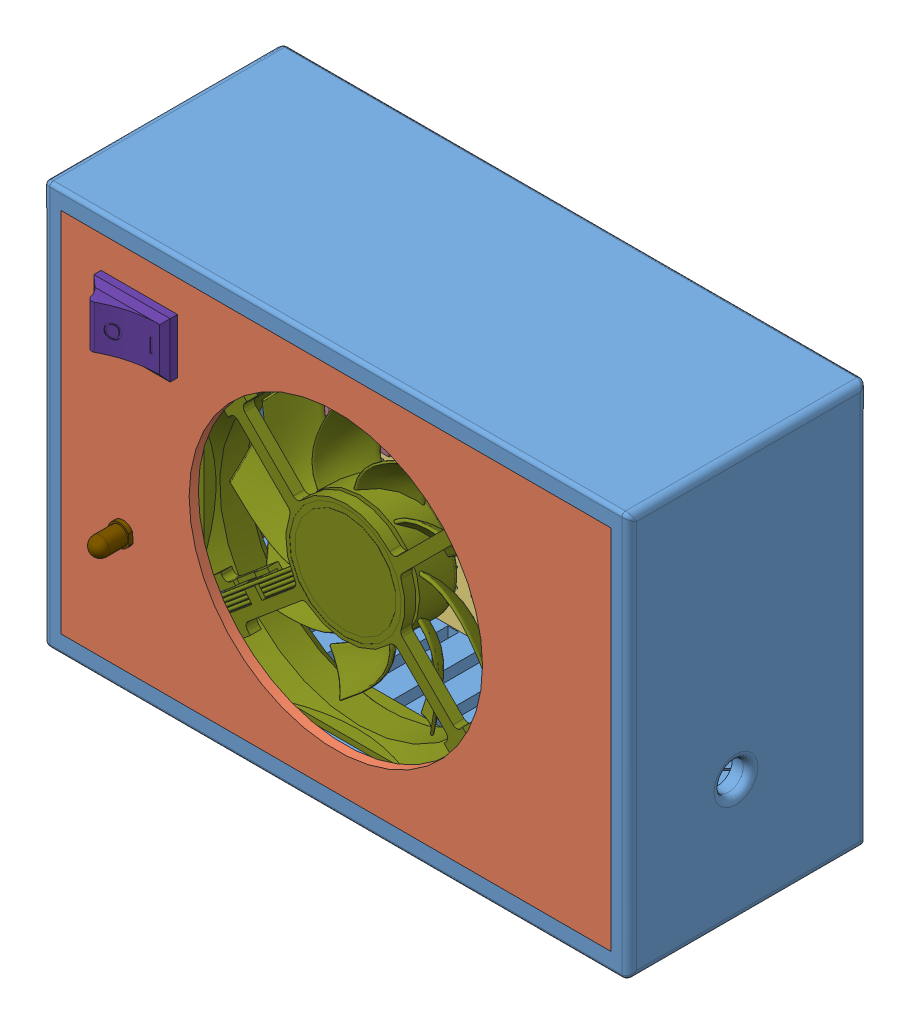
SolidWorks assembly Assem1 final, configuration Default. Lengths in mm. (continued)
Components (placement in the parent): (continued)
- PCB2.step-2: PCB2.step [Default] at (-67.4243 -42.9166 12.1575) size (119 88 45.91) (continued)
  - U5.step-1: U5.step [Default] at origin size (7.89 10.15 6.68) (continued)
    - 5985637968.step-6: 5985637968.step [Default] at (64.2785 40.419 2.66) size (0.64 1 0.27) (continued)
      - Extruded-3.step-1: Extruded-3.step [Default] at origin size (0.64 1 0.27)
    - 5985638128.step-6: 5985638128.step [Default] at (64.466 40.419 -1.6) size (0.27 0.72 1.6)
      - Extruded-2.step-1: Extruded-2.step [Default] at origin size (0.27 0.72 1.6)
    - 5985637808.step-7: 5985637808.step [Default] at (64.466 42.959 0) size (0.27 1 2.66)
      - Extruded-4.step-1: Extruded-4.step [Default] at origin size (0.27 1 2.66)
    - 5985637968.step-7: 5985637968.step [Default] at (64.2785 42.959 2.66) size (0.64 1 0.27)
      - Extruded-3.step-1: Extruded-3.step [Default] at origin size (0.64 1 0.27)
    - 5985638128.step-7: 5985638128.step [Default] at (64.466 42.959 -1.6) size (0.27 0.72 1.6)
      - Extruded-2.step-1: Extruded-2.step [Default] at origin size (0.27 0.72 1.6)
    - 5985637808.step-8: 5985637808.step [Default] at (64.466 45.499 0) size (0.27 1 2.66)
      - Extruded-4.step-1: Extruded-4.step [Default] at origin size (0.27 1 2.66)
    - 5985637968.step-8: 5985637968.step [Default] at (64.2785 45.499 2.66) size (0.64 1 0.27)
      - Extruded-3.step-1: Extruded-3.step [Default] at origin size (0.64 1 0.27)
    - 5985638128.step-8: 5985638128.step [Default] at (64.466 45.499 -1.6) size (0.27 0.72 1.6)
      - Extruded-2.step-1: Extruded-2.step [Default] at origin size (0.27 0.72 1.6)
    - 5985638288.step-1: 5985638288.step [Default] at (60.656 41.689 0.51) size (6.6 10.15 4.57)
      - Extruded-5.step-1: Extruded-5.step [Default] at origin size (6.6 10.15 4.57)
  - U4.step-1: U4.step [Default] at origin size (7.89 10.15 6.68)
    - 5985637808.step-1: 5985637808.step [Default] at (53.163 79.789 0) size (0.27 1 2.66)
      - Extruded-4.step-1: Extruded-4.step [Default] at origin size (0.27 1 2.66)
    - 5985637968.step-1: 5985637968.step [Default] at (53.3505 79.789 2.66) size (0.64 1 0.27)
      - Extruded-3.step-1: Extruded-3.step [Default] at origin size (0.64 1 0.27)
    - 5985638128.step-1: 5985638128.step [Default] at (53.163 79.789 -1.6) size (0.27 0.72 1.6)
      - Extruded-2.step-1: Extruded-2.step [Default] at origin size (0.27 0.72 1.6)
    - 5985637808.step-2: 5985637808.step [Default] at (53.163 77.249 0) size (0.27 1 2.66)
      - Extruded-4.step-1: Extruded-4.step [Default] at origin size (0.27 1 2.66)
    - 5985637968.step-2: 5985637968.step [Default] at (53.3505 77.249 2.66) size (0.64 1 0.27)
      - Extruded-3.step-1: Extruded-3.step [Default] at origin size (0.64 1 0.27)
    - 5985638128.step-2: 5985638128.step [Default] at (53.163 77.249 -1.6) size (0.27 0.72 1.6)
      - Extruded-2.step-1: Extruded-2.step [Default] at origin size (0.27 0.72 1.6)
    - 5985637808.step-3: 5985637808.step [Default] at (53.163 74.709 0) size (0.27 1 2.66)
      - Extruded-4.step-1: Extruded-4.step [Default] at origin size (0.27 1 2.66)
    - 5985637968.step-3: 5985637968.step [Default] at (53.3505 74.709 2.66) size (0.64 1 0.27)
      - Extruded-3.step-1: Extruded-3.step [Default] at origin size (0.64 1 0.27)
    - 5985638128.step-3: 5985638128.step [Default] at (53.163 74.709 -1.6) size (0.27 0.72 1.6)
      - Extruded-2.step-1: Extruded-2.step [Default] at origin size (0.27 0.72 1.6)
    - 5985637808.step-4: 5985637808.step [Default] at (53.163 72.169 0) size (0.27 1 2.66)
      - Extruded-4.step-1: Extruded-4.step [Default] at origin size (0.27 1 2.66)
    - 5985637968.step-4: 5985637968.step [Default] at (53.3505 72.169 2.66) size (0.64 1 0.27)
      - Extruded-3.step-1: Extruded-3.step [Default] at origin size (0.64 1 0.27)
    - 5985638128.step-4: 5985638128.step [Default] at (53.163 72.169 -1.6) size (0.27 0.72 1.6)
      - Extruded-2.step-1: Extruded-2.step [Default] at origin size (0.27 0.72 1.6)
    - 5985637808.step-5: 5985637808.step [Default] at (60.783 72.169 0) size (0.27 1 2.66)
      - Extruded-4.step-1: Extruded-4.step [Default] at origin size (0.27 1 2.66)
    - 5985637968.step-5: 5985637968.step [Default] at (60.5955 72.169 2.66) size (0.64 1 0.27)
      - Extruded-3.step-1: Extruded-3.step [Default] at origin size (0.64 1 0.27)
    - 5985638128.step-5: 5985638128.step [Default] at (60.783 72.169 -1.6) size (0.27 0.72 1.6)
      - Extruded-2.step-1: Extruded-2.step [Default] at origin size (0.27 0.72 1.6)
    - 5985637808.step-6: 5985637808.step [Default] at (60.783 74.709 0) size (0.27 1 2.66)
      - Extruded-4.step-1: Extruded-4.step [Default] at origin size (0.27 1 2.66)
    - 5985637968.step-6: 5985637968.step [Default] at (60.5955 74.709 2.66) size (0.64 1 0.27)
      - Extruded-3.step-1: Extruded-3.step [Default] at origin size (0.64 1 0.27)
    - 5985638128.step-6: 5985638128.step [Default] at (60.783 74.709 -1.6) size (0.27 0.72 1.6)
      - Extruded-2.step-1: Extruded-2.step [Default] at origin size (0.27 0.72 1.6)
    - 5985637808.step-7: 5985637808.step [Default] at (60.783 77.249 0) size (0.27 1 2.66)
      - Extruded-4.step-1: Extruded-4.step [Default] at origin size (0.27 1 2.66)
    - 5985637968.step-7: 5985637968.step [Default] at (60.5955 77.249 2.66) size (0.64 1 0.27)
      - Extruded-3.step-1: Extruded-3.step [Default] at origin size (0.64 1 0.27)
    - 5985638128.step-7: 5985638128.step [Default] at (60.783 77.249 -1.6) size (0.27 0.72 1.6)
      - Extruded-2.step-1: Extruded-2.step [Default] at origin size (0.27 0.72 1.6)
    - 5985637808.step-8: 5985637808.step [Default] at (60.783 79.789 0) size (0.27 1 2.66)
      - Extruded-4.step-1: Extruded-4.step [Default] at origin size (0.27 1 2.66)
    - 5985637968.step-8: 5985637968.step [Default] at (60.5955 79.789 2.66) size (0.64 1 0.27)
      - Extruded-3.step-1: Extruded-3.step [Default] at origin size (0.64 1 0.27)
    - 5985638128.step-8: 5985638128.step [Default] at (60.783 79.789 -1.6) size (0.27 0.72 1.6)
      - Extruded-2.step-1: Extruded-2.step [Default] at origin size (0.27 0.72 1.6)
    - 5985638288.step-1: 5985638288.step [Default] at (56.973 75.979 0.51) size (6.6 10.15 4.57)
      - Extruded-5.step-1: Extruded-5.step [Default] at origin size (6.6 10.15 4.57)
  - U2.step-1: U2.step [Default] at origin size (10.2 4.7 20.55)
    - 5985631488.step-1: 5985631488.step [Default] at (24.334 71.534 0) size (1.52 0.53 3)
      - Extruded-6.step-1: Extruded-6.step [Default] at origin size (1.52 0.53 3)
    - 5985631328.step-1: 5985631328.step [Default] at (24.334 71.534 -1.6) size (0.8 0.53 1.6)
      - Extruded-7.step-1: Extruded-7.step [Default] at origin size (0.8 0.53 1.6)
    - 5985631488.step-2: 5985631488.step [Default] at (26.874 71.534 0) size (1.52 0.53 3)
      - Extruded-6.step-1: Extruded-6.step [Default] at origin size (1.52 0.53 3)
    - 5985631328.step-2: 5985631328.step [Default] at (26.874 71.534 -1.6) size (0.8 0.53 1.6)
      - Extruded-7.step-1: Extruded-7.step [Default] at origin size (0.8 0.53 1.6)
    - 5985631488.step-3: 5985631488.step [Default] at (29.414 71.534 0) size (1.52 0.53 3)
      - Extruded-6.step-1: Extruded-6.step [Default] at origin size (1.52 0.53 3)
    - 5985631328.step-3: 5985631328.step [Default] at (29.414 71.534 -1.6) size (0.8 0.53 1.6)
      - Extruded-7.step-1: Extruded-7.step [Default] at origin size (0.8 0.53 1.6)
    - 5985630848.step-1: 5985630848.step [Default] at (26.874 71.844 3) size (10.2 4.7 9.2)
      - Extruded-8.step-1: Extruded-8.step [Default] at origin size (10.2 4.7 9.2)
    - 5985630688.step-1: 5985630688.step [Default] at (26.874 73.519 12.2) size (9.9 1.35 2.15)
      - Extruded-9.step-1: Extruded-9.step [Default] at origin size (9.9 1.35 2.15)
    - 5985630528.step-1: 5985630528.step [Default] at (24.2234 73.519 14.35) size (4.6 1.35 0.04)
      - Extruded-10.step-1: Extruded-10.step [Default] at origin size (4.6 1.35 0.04)
    - 5985630528.step-2: 5985630528.step [Default] at (29.5246 73.519 14.35) size (4.6 1.35 0.04)
      - Extruded-10.step-1: Extruded-10.step [Default] at origin size (4.6 1.35 0.04)
    - 5985630288.step-1: 5985630288.step [Default] at (24.2234 73.519 17.92) size (4.6 1.35 0.03)
      - Extruded-11.step-1: Extruded-11.step [Default] at origin size (4.6 1.35 0.03)
    - 5985630288.step-2: 5985630288.step [Default] at (29.5246 73.519 17.92) size (4.6 1.35 0.03)
      - Extruded-11.step-1: Extruded-11.step [Default] at origin size (4.6 1.35 0.03)
    - 5985630048.step-1: 5985630048.step [Default] at (24.0546 73.519 14.38) size (4.26 1.35 0.11)
      - Extruded-12.step-1: Extruded-12.step [Default] at origin size (4.26 1.35 0.11)
    - 5985630048.step-2: 5985630048.step [Default] at (29.6934 73.519 14.38) size (4.26 1.35 0.11)
      - Extruded-12.step-1: Extruded-12.step [Default] at origin size (4.26 1.35 0.11)
    - 5985630048.step-3: 5985630048.step [Default] at (24.0546 73.519 17.81) size (4.26 1.35 0.11)
      - Extruded-12.step-1: Extruded-12.step [Default] at origin size (4.26 1.35 0.11)
    - 5985630048.step-4: 5985630048.step [Default] at (29.6934 73.519 17.81) size (4.26 1.35 0.11)
      - Extruded-12.step-1: Extruded-12.step [Default] at origin size (4.26 1.35 0.11)
    - 5985629648.step-1: 5985629648.step [Default] at (23.899 73.519 14.49) size (3.95 1.35 0.17)
      - Extruded-13.step-1: Extruded-13.step [Default] at origin size (3.95 1.35 0.17)
    - 5985629648.step-2: 5985629648.step [Default] at (29.849 73.519 14.49) size (3.95 1.35 0.17)
      - Extruded-13.step-1: Extruded-13.step [Default] at origin size (3.95 1.35 0.17)
    - 5985629408.step-1: 5985629408.step [Default] at (23.899 73.519 17.65) size (3.95 1.35 0.17)
      - Extruded-14.step-1: Extruded-14.step [Default] at origin size (3.95 1.35 0.17)
    - 5985629408.step-2: 5985629408.step [Default] at (29.849 73.519 17.65) size (3.95 1.35 0.17)
      - Extruded-14.step-1: Extruded-14.step [Default] at origin size (3.95 1.35 0.17)
    - 5985629168.step-1: 5985629168.step [Default] at (23.7626 73.519 14.65) size (3.68 1.35 0.23)
      - Extruded-15.step-1: Extruded-15.step [Default] at origin size (3.68 1.35 0.23)
    - 5985629168.step-2: 5985629168.step [Default] at (29.9854 73.519 14.65) size (3.68 1.35 0.23)
      - Extruded-15.step-1: Extruded-15.step [Default] at origin size (3.68 1.35 0.23)
    - 5985629168.step-3: 5985629168.step [Default] at (23.7626 73.519 17.42) size (3.68 1.35 0.23)
      - Extruded-15.step-1: Extruded-15.step [Default] at origin size (3.68 1.35 0.23)
    - 5985629168.step-4: 5985629168.step [Default] at (29.9854 73.519 17.42) size (3.68 1.35 0.23)
      - Extruded-15.step-1: Extruded-15.step [Default] at origin size (3.68 1.35 0.23)
    - 5985628768.step-1: 5985628768.step [Default] at (23.6507 73.519 14.88) size (3.45 1.35 0.27)
      - Extruded-16.step-1: Extruded-16.step [Default] at origin size (3.45 1.35 0.27)
    - 5985628768.step-2: 5985628768.step [Default] at (30.0973 73.519 14.88) size (3.45 1.35 0.27)
      - Extruded-16.step-1: Extruded-16.step [Default] at origin size (3.45 1.35 0.27)
    - 5985628528.step-1: 5985628528.step [Default] at (23.6507 73.519 17.15) size (3.45 1.35 0.28)
      - Extruded-17.step-1: Extruded-17.step [Default] at origin size (3.45 1.35 0.28)
    - 5985628528.step-2: 5985628528.step [Default] at (30.0973 73.519 17.15) size (3.45 1.35 0.28)
      - Extruded-17.step-1: Extruded-17.step [Default] at origin size (3.45 1.35 0.28)
    - 5985628288.step-1: 5985628288.step [Default] at (23.5675 73.519 15.15) size (3.29 1.35 0.32)
      - Extruded-18.step-1: Extruded-18.step [Default] at origin size (3.29 1.35 0.32)
    - 5985628288.step-2: 5985628288.step [Default] at (30.1805 73.519 15.15) size (3.29 1.35 0.32)
      - Extruded-18.step-1: Extruded-18.step [Default] at origin size (3.29 1.35 0.32)
    - 5985628048.step-1: 5985628048.step [Default] at (23.5675 73.519 16.84) size (3.29 1.35 0.32)
      - Extruded-19.step-1: Extruded-19.step [Default] at origin size (3.29 1.35 0.32)
    - 5985628048.step-2: 5985628048.step [Default] at (30.1805 73.519 16.84) size (3.29 1.35 0.32)
      - Extruded-19.step-1: Extruded-19.step [Default] at origin size (3.29 1.35 0.32)
    - 5985627808.step-1: 5985627808.step [Default] at (23.5163 73.519 15.46) size (3.18 1.35 0.34)
      - Extruded-20.step-1: Extruded-20.step [Default] at origin size (3.18 1.35 0.34)
    - 5985627808.step-2: 5985627808.step [Default] at (30.2317 73.519 15.46) size (3.18 1.35 0.34)
      - Extruded-20.step-1: Extruded-20.step [Default] at origin size (3.18 1.35 0.34)
    - 5985627808.step-3: 5985627808.step [Default] at (23.5163 73.519 16.5) size (3.18 1.35 0.34)
      - Extruded-20.step-1: Extruded-20.step [Default] at origin size (3.18 1.35 0.34)
    - 5985627808.step-4: 5985627808.step [Default] at (30.2317 73.519 16.5) size (3.18 1.35 0.34)
      - Extruded-20.step-1: Extruded-20.step [Default] at origin size (3.18 1.35 0.34)
    - 5985063680.step-1: 5985063680.step [Default] at (23.499 73.519 15.8) size (3.15 1.35 0.35)
      - Extruded-21.step-1: Extruded-21.step [Default] at origin size (3.15 1.35 0.35)
    - 5985063680.step-2: 5985063680.step [Default] at (30.249 73.519 15.8) size (3.15 1.35 0.35)
      - Extruded-21.step-1: Extruded-21.step [Default] at origin size (3.15 1.35 0.35)
    - 5985063440.step-1: 5985063440.step [Default] at (23.499 73.519 16.15) size (3.15 1.35 0.36)
      - Extruded-22.step-1: Extruded-22.step [Default] at origin size (3.15 1.35 0.36)
    - 5985063440.step-2: 5985063440.step [Default] at (30.249 73.519 16.15) size (3.15 1.35 0.36)
      - Extruded-22.step-1: Extruded-22.step [Default] at origin size (3.15 1.35 0.36)
    - 5985063200.step-1: 5985063200.step [Default] at (26.874 73.519 17.95) size (9.9 1.35 1)
      - Extruded-23.step-1: Extruded-23.step [Default] at origin size (9.9 1.35 1)
  - U1.step-1: U1.step [Default] at origin size (10.5 4.7 16.2)
    - 5985631808.step-1: 5985631808.step [Default] at (11.754 60.146 3.5) size (10.5 4.7 9.55)
      - Extruded-24.step-1: Extruded-24.step [Default] at origin size (10.5 4.7 9.55)
    - 5985631648.step-1: 5985631648.step [Default] at (11.754 61.796 13.05) size (10.4 1.3 6.65)
      - Extruded-25.step-1: Extruded-25.step [Default] at origin size (10.4 1.3 6.65)
  - R6_A.step-1: R6_A.step [Default] at origin size (9.5 29.91 14)
    - Res_Yageo_SQP500JB-1R2_eec.step-1: Res_Yageo_SQP500JB-1R2_eec.step [Default] at (99 68 0) x (0 1 0) z (0 0 1) size (29.91 9.5 14)
      - 1.step-1: 1.step [Default] at origin size (29.91 0.8 9.4)
      - 2.step-1: 2.step [Default] at origin size (22 9.5 10)
      - Yageo_Logo.step-1: Yageo_Logo.step [Default] at (-8.1443 3.6121 9.991) size (4.52 1.05 0.01)
  - Q2.step-1: Q2.step [Default] at origin size (10.3 4.85 21.45)
    - 5985059040.step-1: 5985059040.step [Default] at (85.019 64.409 18.98) size (9.95 1.25 0.87)
      - Extruded-26.step-1: Extruded-26.step [Default] at origin size (9.95 1.25 0.87)
    - 5985058880.step-1: 5985058880.step [Default] at (81.569 64.409 17.05) size (3.05 1.25 0.38)
      - Extruded-27.step-1: Extruded-27.step [Default] at origin size (3.05 1.25 0.38)
    - 5985058880.step-2: 5985058880.step [Default] at (88.469 64.409 17.05) size (3.05 1.25 0.38)
      - Extruded-27.step-1: Extruded-27.step [Default] at origin size (3.05 1.25 0.38)
    - 5985058640.step-1: 5985058640.step [Default] at (81.569 64.409 16.67) size (3.05 1.25 0.38)
      - Extruded-28.step-1: Extruded-28.step [Default] at origin size (3.05 1.25 0.38)
    - 5985058640.step-2: 5985058640.step [Default] at (88.469 64.409 16.67) size (3.05 1.25 0.38)
      - Extruded-28.step-1: Extruded-28.step [Default] at origin size (3.05 1.25 0.38)
    - 5985058400.step-1: 5985058400.step [Default] at (81.5875 64.409 17.43) size (3.09 1.25 0.36)
      - Extruded-29.step-1: Extruded-29.step [Default] at origin size (3.09 1.25 0.36)
    - 5985058400.step-2: 5985058400.step [Default] at (88.4505 64.409 17.43) size (3.09 1.25 0.36)
      - Extruded-29.step-1: Extruded-29.step [Default] at origin size (3.09 1.25 0.36)
    - 5985058160.step-1: 5985058160.step [Default] at (81.5875 64.409 16.31) size (3.09 1.25 0.37)
      - Extruded-30.step-1: Extruded-30.step [Default] at origin size (3.09 1.25 0.37)
    - 5985058160.step-2: 5985058160.step [Default] at (88.4505 64.409 16.31) size (3.09 1.25 0.37)
      - Extruded-30.step-1: Extruded-30.step [Default] at origin size (3.09 1.25 0.37)
    - 5985057920.step-1: 5985057920.step [Default] at (81.6423 64.409 17.79) size (3.2 1.25 0.33)
      - Extruded-31.step-1: Extruded-31.step [Default] at origin size (3.2 1.25 0.33)
    - 5985057920.step-2: 5985057920.step [Default] at (88.3957 64.409 17.79) size (3.2 1.25 0.33)
      - Extruded-31.step-1: Extruded-31.step [Default] at origin size (3.2 1.25 0.33)
    - 5985057680.step-1: 5985057680.step [Default] at (81.6423 64.409 15.98) size (3.2 1.25 0.34)
      - Extruded-32.step-1: Extruded-32.step [Default] at origin size (3.2 1.25 0.34)
    - 5985057680.step-2: 5985057680.step [Default] at (88.3957 64.409 15.98) size (3.2 1.25 0.34)
      - Extruded-32.step-1: Extruded-32.step [Default] at origin size (3.2 1.25 0.34)
    - 5985057440.step-1: 5985057440.step [Default] at (81.7312 64.409 18.12) size (3.37 1.25 0.3)
      - Extruded-33.step-1: Extruded-33.step [Default] at origin size (3.37 1.25 0.3)
    - 5985057440.step-2: 5985057440.step [Default] at (88.3068 64.409 18.12) size (3.37 1.25 0.3)
      - Extruded-33.step-1: Extruded-33.step [Default] at origin size (3.37 1.25 0.3)
    - 5985057440.step-3: 5985057440.step [Default] at (81.7312 64.409 15.69) size (3.37 1.25 0.3)
      - Extruded-33.step-1: Extruded-33.step [Default] at origin size (3.37 1.25 0.3)
    - 5985057440.step-4: 5985057440.step [Default] at (88.3068 64.409 15.69) size (3.37 1.25 0.3)
      - Extruded-33.step-1: Extruded-33.step [Default] at origin size (3.37 1.25 0.3)
    - 5985057040.step-1: 5985057040.step [Default] at (81.8509 64.409 18.41) size (3.61 1.25 0.25)
      - Extruded-34.step-1: Extruded-34.step [Default] at origin size (3.61 1.25 0.25)
    - 5985057040.step-2: 5985057040.step [Default] at (88.1871 64.409 18.41) size (3.61 1.25 0.25)
      - Extruded-34.step-1: Extruded-34.step [Default] at origin size (3.61 1.25 0.25)
    - 5985056800.step-1: 5985056800.step [Default] at (81.8509 64.409 15.45) size (3.61 1.25 0.24)
      - Extruded-35.step-1: Extruded-35.step [Default] at origin size (3.61 1.25 0.24)
    - 5985056800.step-2: 5985056800.step [Default] at (88.1871 64.409 15.45) size (3.61 1.25 0.24)
      - Extruded-35.step-1: Extruded-35.step [Default] at origin size (3.61 1.25 0.24)
    - 5985056560.step-1: 5985056560.step [Default] at (81.9968 64.409 18.65) size (3.91 1.25 0.18)
      - Extruded-36.step-1: Extruded-36.step [Default] at origin size (3.91 1.25 0.18)
    - 5985056560.step-2: 5985056560.step [Default] at (88.0412 64.409 18.65) size (3.91 1.25 0.18)
      - Extruded-36.step-1: Extruded-36.step [Default] at origin size (3.91 1.25 0.18)
    - 5985056560.step-3: 5985056560.step [Default] at (81.9968 64.409 15.27) size (3.91 1.25 0.18)
      - Extruded-36.step-1: Extruded-36.step [Default] at origin size (3.91 1.25 0.18)
    - 5985056560.step-4: 5985056560.step [Default] at (88.0412 64.409 15.27) size (3.91 1.25 0.18)
      - Extruded-36.step-1: Extruded-36.step [Default] at origin size (3.91 1.25 0.18)
    - 5985056160.step-1: 5985056160.step [Default] at (82.1632 64.409 18.83) size (4.24 1.25 0.11)
      - Extruded-37.step-1: Extruded-37.step [Default] at origin size (4.24 1.25 0.11)
    - 5985056160.step-2: 5985056160.step [Default] at (87.8748 64.409 18.83) size (4.24 1.25 0.11)
      - Extruded-37.step-1: Extruded-37.step [Default] at origin size (4.24 1.25 0.11)
    - 5985055920.step-1: 5985055920.step [Default] at (82.1632 64.409 15.16) size (4.24 1.25 0.12)
      - Extruded-38.step-1: Extruded-38.step [Default] at origin size (4.24 1.25 0.12)
    - 5985055920.step-2: 5985055920.step [Default] at (87.8748 64.409 15.16) size (4.24 1.25 0.12)
      - Extruded-38.step-1: Extruded-38.step [Default] at origin size (4.24 1.25 0.12)
    - 5985055680.step-1: 5985055680.step [Default] at (82.3437 64.409 18.94) size (4.6 1.25 0.04)
      - Extruded-39.step-1: Extruded-39.step [Default] at origin size (4.6 1.25 0.04)
    - 5985055680.step-2: 5985055680.step [Default] at (87.6943 64.409 18.94) size (4.6 1.25 0.04)
      - Extruded-39.step-1: Extruded-39.step [Default] at origin size (4.6 1.25 0.04)
    - 5985055680.step-3: 5985055680.step [Default] at (82.3437 64.409 15.13) size (4.6 1.25 0.04)
      - Extruded-39.step-1: Extruded-39.step [Default] at origin size (4.6 1.25 0.04)
    - 5985055680.step-4: 5985055680.step [Default] at (87.6943 64.409 15.13) size (4.6 1.25 0.04)
      - Extruded-39.step-1: Extruded-39.step [Default] at origin size (4.6 1.25 0.04)
    - 5985055280.step-1: 5985055280.step [Default] at (85.019 64.409 13.65) size (9.95 1.25 1.48)
      - Extruded-40.step-1: Extruded-40.step [Default] at origin size (9.95 1.25 1.48)
    - 5985055120.step-1: 5985055120.step [Default] at (85.019 66.209 2.8) size (10.3 4.85 10.85)
      - Extruded-41.step-1: Extruded-41.step [Default] at origin size (10.3 4.85 10.85)
    - 5985054960.step-1: 5985054960.step [Default] at (82.479 66.454 -1.6) size (0.78 0.5 1.6)
      - Extruded-42.step-1: Extruded-42.step [Default] at origin size (0.78 0.5 1.6)
    - 5985054800.step-1: 5985054800.step [Default] at (82.479 66.454 0) size (1.34 0.5 2.8)
      - Extruded-43.step-1: Extruded-43.step [Default] at origin size (1.34 0.5 2.8)
    - 5985054960.step-2: 5985054960.step [Default] at (85.019 66.454 -1.6) size (0.78 0.5 1.6)
      - Extruded-42.step-1: Extruded-42.step [Default] at origin size (0.78 0.5 1.6)
    - 5985054800.step-2: 5985054800.step [Default] at (85.019 66.454 0) size (1.34 0.5 2.8)
      - Extruded-43.step-1: Extruded-43.step [Default] at origin size (1.34 0.5 2.8)
    - 5985054960.step-3: 5985054960.step [Default] at (87.559 66.454 -1.6) size (0.78 0.5 1.6)
      - Extruded-42.step-1: Extruded-42.step [Default] at origin size (0.78 0.5 1.6)
    - 5985054800.step-3: 5985054800.step [Default] at (87.559 66.454 0) size (1.34 0.5 2.8)
      - Extruded-43.step-1: Extruded-43.step [Default] at origin size (1.34 0.5 2.8)
  - Q1.step-1: Q1.step [Default] at origin size (4.76 3.61 5.33)
    - 6657494432.step-1: 6657494432.step [Default] at (71.73 58.4075 0) size (4.76 3.61 5.33)
      - Extruded-44.step-1: Extruded-44.step [Default] at origin size (4.76 3.61 5.33)
  - L1.step-1: L1.step [Default] at origin size (11.74 11.74 10.5)
    - 744741102.step-1: 744741102.step [Default] at (84.0144 31.9866 1) x (0.707107 -0.707107 0) z (0 0 1) size (8.3 8.3 10.5)
      - Kern.step-1: Kern.step [Default] at origin size (6.7 4.46 3.58)
      - Kern-45.step-1: Kern-45.step [Default] at origin size (7.95 8 5.53)
      - Pin.step-1: Pin.step [Default] at (1.7678 -1.7678 0.9) size (1 1 6.9)
      - Pin.step-2: Pin.step [Default] at (-1.7678 1.7678 0.9) x (0.981852 -0.189648 0) z (0 0 1) size (1 1 6.9)
      - Mantel.step-1: Mantel.step [Default] at (0 0 2.25) size (8.3 8.3 4.5)
  - J2.step-1: J2.step [Default] at origin size (10.73 8.1 13.5)
    - 1729128.step-1: 1729128.step [Default] at (78.2391 5.5731 0.0128) x (0 -1 0) z (-1 0 0) size (8.1 13.5 10.73)
      - mkdsn_1.5-2-5.08.step-1: mkdsn_1.5-2-5.08.step [Default] at (-39.331 -15.5089 -8.19) x (-1 0 0) z (0 0 -1) size (8.1 13.5 10.73)
  - J1.step-1: J1.step [Default] at origin size (10.73 8.1 13.5)
    - 1729128.step-1: 1729128.step [Default] at (17.2839 80.8529 0.0128) x (0 1 0) z (1 0 0) size (8.1 13.5 10.73)
      - mkdsn_1.5-2-5.08.step-1: mkdsn_1.5-2-5.08.step [Default] at (-39.331 -15.5089 -8.19) x (-1 0 0) z (0 0 -1) size (8.1 13.5 10.73)
  - C7.step-1: C7.step [Default] at origin size (8.5 8.5 12.5)
    - 5985638368.step-1: 5985638368.step [Default] at (84 21 0) size (8.5 8.5 12.5)
      - Extruded-46.step-1: Extruded-46.step [Default] at origin size (8.5 8.5 12.5)
  - Free-Models.step-1: Free-Models.step [Default] at origin size (90.22 11.92 20)
    - HeatsinkTO220NoScrew.step-1: HeatsinkTO220NoScrew.step [Default] at (84.8 57.7 1) x (1 0 0) z (0 0 1) size (15 11 20)
      - HeatSink.step-1: HeatSink.step [Default] at origin size (15 11 20)
    - TO220_Heatsink_RGB12040119.step-1: TO220_Heatsink_RGB12040119.step [Default] at (2.075 64 1) x (1 0 0) z (0 0 -1) size (19.05 9.53 19.05)
- Exhaust Fan 80mm x 80mm x 15mm -1: Exhaust Fan 80mm x 80mm x 15mm  [Default] at (0.1185 0.8013 50) x (1 0 0) z (0 1 0) size (80 21.83 80)
- Square Rocker Switch v2.step-1: Square Rocker Switch v2.step [Default] at (-53.5954 33.8201 60) size (20.83 14.99 24.27)
- red-led-5mm-1: red-led-5mm [Default] at (-58.0002 -17.6048 60.575) x (0.056945 -0.998377 0) z (0 0 1) size (5.95 5.62 28.7)
Mates (geometry in assembly coordinates):
- Concentric2: concentric anti-aligned: cylinder of PCB2.step-2/Board.step-1/Open CASCADE STEP translator 6.8 2.1.1.step-1 through (-64.4243 42.0834 11.746) axis (0 0 -1) radius 1.25; circle of Lead acid charger_enclosure-2
- Coincident43: coincident aligned: plane of Lead acid charger_enclosure-2; plane of PCB2.step-2/Board.step-1/Open CASCADE STEP translator 6.8 2.1.1.step-1 through (-67.4243 -42.9166 11.746) normal (0 0 -1)
- Parallel13: parallel: line of Lead acid charger_enclosure-2 through (78 -54 60) axis (0 1 0); plane of Part2-3 through (0 0 60) normal (0 0 1)
- Parallel16: parallel aligned: plane of Lead acid charger_enclosure-2 through (0 0 0) normal (0 0 1); plane of Part2-3 through (0 0 60) normal (0 0 1)
- Parallel23: parallel aligned: plane of Lead acid charger_enclosure-2 through (-75 55 60) normal (0 1 0); plane of Part2-3 through (75 50 57.5) normal (0 1 0)
- Parallel25: parallel aligned: plane of Lead acid charger_enclosure-2 through (0 0 -5) normal (0 0 -1); plane of Part2-3 through (0 0 57.5) normal (0 0 -1)
- Parallel26: parallel aligned: plane of Lead acid charger_enclosure-2 through (-80 50 60) normal (-1 0 0); plane of Part2-3 through (-75 50 57.5) normal (-1 0 0)
- Parallel27: parallel aligned: plane of Lead acid charger_enclosure-2 through (-75 -55 60) normal (0 -1 0); plane of Part2-3 through (75 -50 57.5) normal (0 -1 0)
- Coincident79: coincident anti-aligned: line of Lead acid charger_enclosure-2 through (75 -50 60) axis (0 1 0); line of Part2-3 through (75 50 60) axis (0 -1 0)
- Coincident81: coincident anti-aligned: line of Lead acid charger_enclosure-2 through (-75 -50 60) axis (1 0 0); line of Part2-3 through (75 -50 60) axis (-1 0 0)
- Coincident82: coincident anti-aligned: plane of Part2-3 through (0 0 57.5) normal (0 0 -1); plane of Exhaust Fan 80mm x 80mm x 15mm -1 through (0.1185 0.8013 57.5) normal (0 0 1)
- Coincident83: coincident anti-aligned: circle of Part2-3; plane of Exhaust Fan 80mm x 80mm x 15mm -1 through (0.1185 0.8013 57.5) normal (0 0 1)
- Tangent2: tangent: circle of Part2-3; plane of Exhaust Fan 80mm x 80mm x 15mm -1 through (0.1185 0.8013 57.5) normal (0 0 1)
- Parallel28: parallel anti-aligned: plane of Part2-3 through (0 0 60) normal (0 0 1); plane of Square Rocker Switch v2.step-1 through (-53.5954 33.8201 60) normal (0 0 -1)
- Coincident88: coincident anti-aligned: line of Part2-3 through (-43.1814 26.3271 60) axis (0 1 0); line of Square Rocker Switch v2.step-1 through (-43.1814 41.3131 60) axis (0 -1 0)
- Coincident89: coincident: point of Part2-3; moEndPointRef_w of Square Rocker Switch v2.step-1
- Coincident90: coincident aligned: plane of Part2-3 through (0 0 60) normal (0 0 1); circle of red-led-5mm-1
- Concentric9: concentric aligned: circle of Part2-3; circle of red-led-5mm-1
